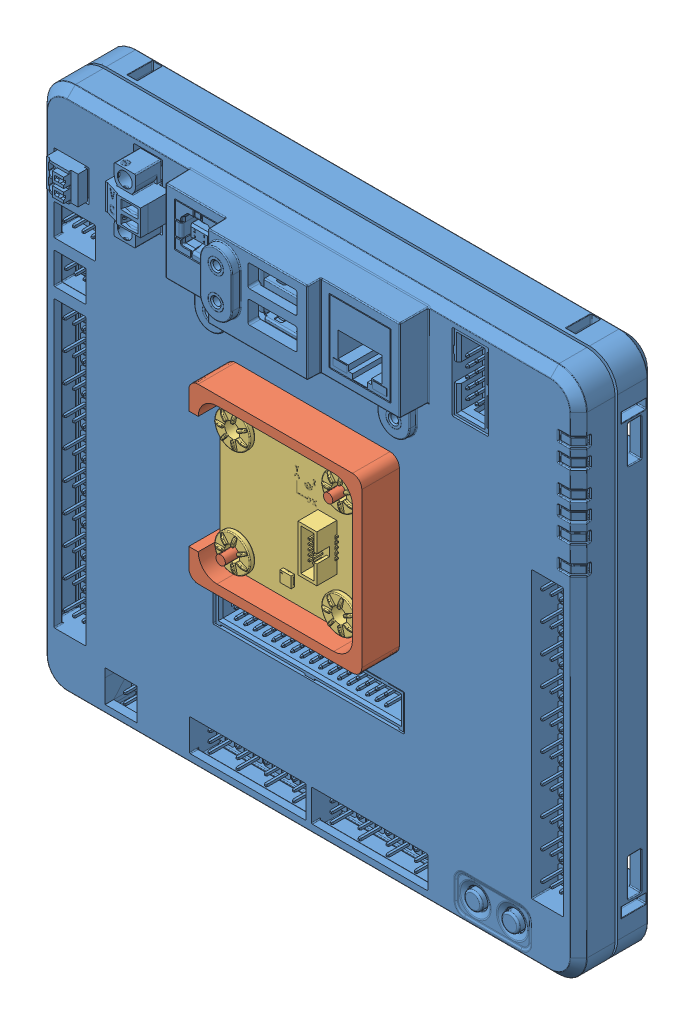
SolidWorks assembly electronics_assembly, configuration Default. Lengths in mm.
Overall size (146.27 143.19 34.5).
4 component instances, 3 part files, 2 mates.
Components (placement in the parent):
- cd_roborio-1: cd_roborio [Default] at (41.2032 69.7642 116.2546) size (146.27 143.19 34.5)
- pigeon enclosure assembly-1: pigeon enclosure assembly [Default] at (65.7618 100.1556 127.512) x (0 -1 0) z (0 0 -1) size (46.86 46.86 11.32)
  - PigeonImuBox-1: PigeonImuBox [Default] at (23.4315 23.4315 0) x (1 0 0) z (0 0 -1) size (46.86 46.86 10.16)
  - PIGEON-1: PIGEON [Default] at (23.749 23.749 -4.1275) x (-1 0 0) z (0 0 -1) size (38.61 38.61 9.36)
Mates (geometry in assembly coordinates):
- Coincident1: coincident anti-aligned: plane of cd_roborio-1 through (41.2032 69.7642 127.512) normal (0 0 1); plane of pigeon enclosure assembly-1/PigeonImuBox-1 through (42.3303 76.7241 127.512) normal (0 0 -1)
- Parallel1: parallel aligned: plane of cd_roborio-1 through (-24.2526 -1.8257 110.0312) normal (0 -1 0); plane of pigeon enclosure assembly-1/PigeonImuBox-1 through (42.3303 53.2926 137.672) normal (0 -1 0)
